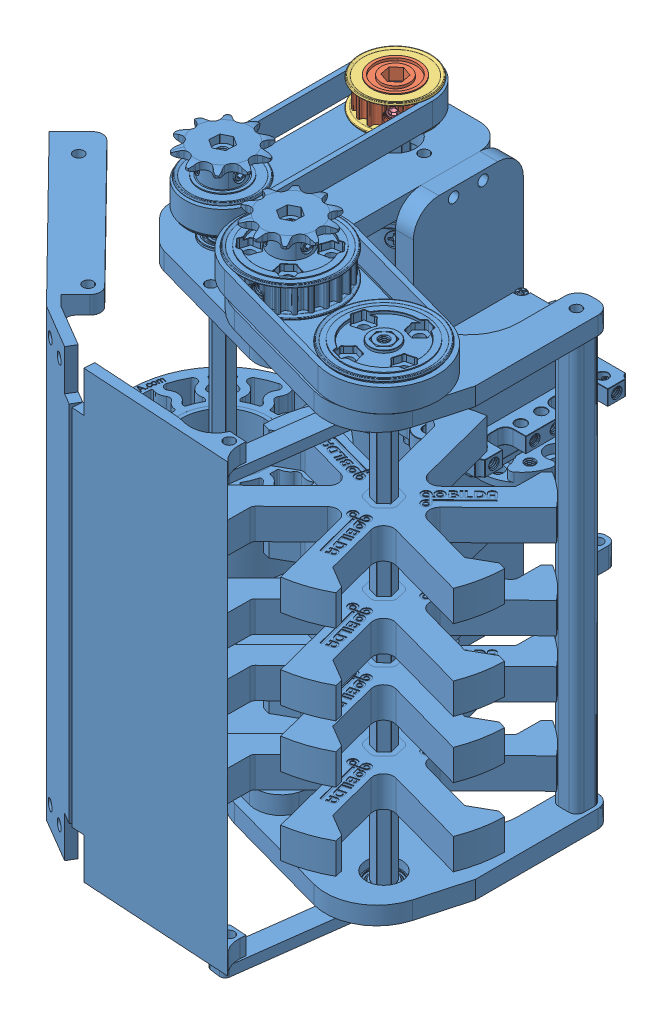
SolidWorks assembly Intake Sub-Assembly League Meet 2, configuration Default. Lengths in mm.
Overall size (196.76 202.81 175.95).
7 component instances, 4 part files, 5 mates.
Components (placement in the parent):
- Intake Sub-Assembly League Meet 2-1: Intake Sub-Assembly League Meet 2 [Default] at (-402.2455 -149.4064 -587.2362) size (196.76 202.81 181.57)
- 5mm timing belt small.STEP-1: 5mm timing belt small.STEP [Default] at (-33.9953 48.0996 -52.8475) x (0 -1 0) z (-0.656331 0 -0.754473) size (12 36.28 36.28)
  - 3417-4008-0016 body.STEP-1: 3417-4008-0016 body.STEP [Default] at (-48.3715 -1.462 -4.6135) size (12 23.97 23.97)
  - 3417-4008-0016 ring.STEP-1: 3417-4008-0016 ring.STEP [Default] at (-36.4912 12.03 13.6144) x (0 -0.999884 -0.015253) z (0 -0.015253 0.999884) size (27.96 1.38 27.96)
  - 3417-4008-0016 ring.STEP-2: 3417-4008-0016 ring.STEP [Default] at (-45.7412 12.03 13.6144) x (0 -0.367708 0.929941) z (0 -0.929941 -0.367708) size (27.96 1.38 27.96)
  - 2806-0005-0006_91390A118.STEP-1: 2806-0005-0006_91390A118.STEP [Default] at (-41.1162 6.0444 17.0702) x (0.62343 -0.390939 -0.677127) z (0 -0.866025 0.5) size (5.01 5.01 6.01)
  - 2806-0005-0006_91390A118.STEP-2: 2806-0005-0006_91390A118.STEP [Default] at (-41.1162 12.03 6.7028) x (0.62343 0.781879 0) z (0 0 -1) size (5.01 5.01 6.01)
Mates (geometry in assembly coordinates):
- Concentric1: concentric anti-aligned: circle of Intake Sub-Assembly League Meet 2 and 3-1; circle of 5mm timing belt small.STEP-1/3417-4008-0016 ring.STEP-1
- Coincident1: coincident aligned: plane of Intake Sub-Assembly League Meet 2-1 through (-52.0071 94.8409 12.2787) normal (0 1 0); plane of 5mm timing belt small.STEP-1/3417-4008-0016 ring.STEP-2 through (-52.0071 94.8409 -55.2235) normal (0 1 0)
- Coincident2: coincident anti-aligned: plane of Intake Sub-Assembly League Meet 2-1 through (-53.1454 65.2159 -51.9138) normal (-0.325227 0 0.945636); plane of 5mm timing belt small.STEP-1/3417-4008-0016 body.STEP-1 through (-51.2345 95.2159 -51.2566) normal (0.325227 0 -0.945636)
- Parallel1: parallel: plane of assembly through (0 0 0) normal (1 0 0); plane of Intake Sub-Assembly League Meet 2-1 through (-30.5071 67.2159 77.6761) normal (1 0 0); plane of assembly
- Parallel2: parallel: plane of assembly through (0 0 0) normal (0 1 0); plane of Intake Sub-Assembly League Meet 2-1 through (-19.8427 74.2159 77.6761) normal (0 1 0); plane of assembly
